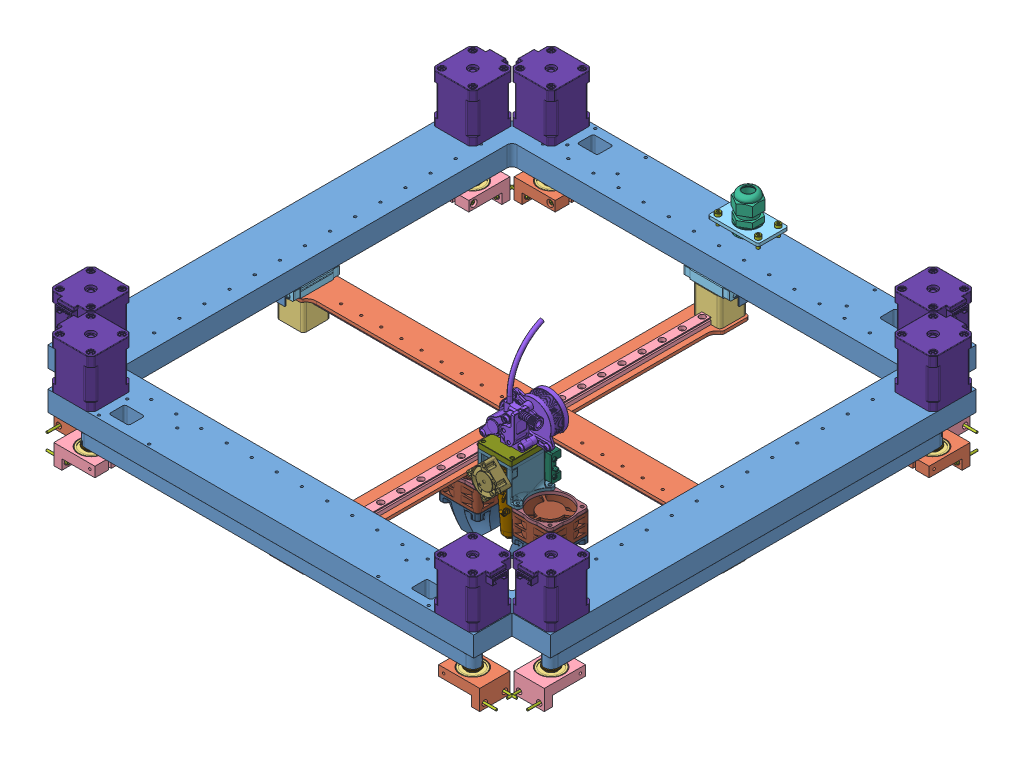
SolidWorks assembly ASM_Gantry_V3, configuration Default. Lengths in mm.
Overall size (500 178.35 500).
200 component instances, 28 part files, 43 mates.
Components (placement in the parent):
- PRT_Gantry_Main_Plate_V4-1: PRT_Gantry_Main_Plate_V4 [Default] at origin size (500 20 500)
- ASM_X_Beam_V1-3: ASM_X_Beam_V1 [Default] at (121.4512 212.7564 -330.8923) x (-1 0 0) z (0 0 1) size (442 41 48.55)
  - PRT_XY_Backer_V1-1: PRT_XY_Backer_V1 [Default] at (121.4512 223.2564 340.8937) size (442 3 38.2)
  - PRT_temp_backer_spacer-1: PRT_temp_backer_spacer [Default] at (328.9512 226.2564 330.8937) size (27 28 27)
  - PRT_temp_backer_spacer-2: PRT_temp_backer_spacer [Default] at (-86.0488 226.2564 330.8937) size (27 28 27)
  - PRT_MGN9H_Rail-2: PRT_MGN9H_Rail [400] at (-78.5488 229.5064 330.8937) x (0 0 -1) z (1 0 0) size (9 6.5 400)
  - PRT_MGN12H_Carriage-1: PRT_MGN12H_Carriage [Default] at (-86.0488 210.2564 314.6937) size (27 10 50.47)
  - PRT_MGN12H_Carriage-2: PRT_MGN12H_Carriage [Default] at (328.9512 210.2564 314.6937) size (27 10 50.47)
- ASM_Y_Beam_V1-1: ASM_Y_Beam_V1 [Default] at (-331.4877 -264.7564 121.4512) x (0 0 -1) z (1 0 0) size (442 41 48.55)
  - PRT_XY_Backer_V1-1: PRT_XY_Backer_V1 [Default] at (121.4512 223.2564 340.8937) size (442 3 38.2)
  - PRT_temp_backer_spacer-1: PRT_temp_backer_spacer [Default] at (328.9512 226.2564 330.8937) size (27 28 27)
  - PRT_temp_backer_spacer-2: PRT_temp_backer_spacer [Default] at (-86.0488 226.2564 330.8937) size (27 28 27)
  - PRT_MGN9H_Rail-2: PRT_MGN9H_Rail [400] at (-78.5488 229.5064 330.8937) x (0 0 -1) z (1 0 0) size (9 6.5 400)
  - PRT_MGN12H_Carriage-1: PRT_MGN12H_Carriage [Default] at (-86.0488 267.2564 314.6937) x (-1 0 0) z (0 0 1) size (27 10 50.47)
  - PRT_MGN12H_Carriage-2: PRT_MGN12H_Carriage [Default] at (328.9512 267.2564 314.6937) x (-1 0 0) z (0 0 1) size (27 10 50.47)
- ASM_Temp_Printhead_V1-1: ASM_Temp_Printhead_V1 [Default] at (-0.594 -28.5 21.5015) x (0 0 -1) z (1 0 0) size (54.33 135.01 54.33) (hidden)
  - PRT_Temp_Printhead_Plate_V1-1: PRT_Temp_Printhead_Plate_V1 [Default] at origin size (47 3 47)
  - PRT_MGN9H_Carriage-1: PRT_MGN9H_Carriage [По умолчанию] at (0 -4 0) x (0 0 1) z (-1 0 0) size (20 8 40.67)
  - PRT_MGN9H_Carriage-2: PRT_MGN9H_Carriage [По умолчанию] at (21.5 7 21.5) x (-1 0 0) z (0 0 1) size (20 8 40.67)
  - PRT_Chube_Integration-1: PRT_Chube_Integration [Default] at (-0.75 -32 22.25) x (1 0 0) z (0 -1 0) size (25.9 25.9 66.25)
  - PRT_Chube_Integration-2: PRT_Chube_Integration [Default] at (-0.75 35 22.25) x (-1 0 0) z (0 1 0) size (25.9 25.9 66.25) (hidden)
- ASM_MGN12_and_Screws_V1-1: ASM_MGN12_and_Screws_V1 [Default] at (35.6885 266.2419 374.1962) x (1 0 0) z (0 0 -1) size (12 14.5 360)
  - PRT_MGN12H_Rail-1: PRT_MGN12H_Rail [Default] at (165.8115 263.7419 208.1962) size (12 8 360)
  - socket head cap screw_am-1: socket head cap screw_am [B18.3.1M - 3 x 0.5 x 10 Hex SHCS -- 10NHX] at (171.8115 270.2419 550.6962) x (0 -1 0) z (0 0 1) size (13 5.5 5.5)
  - socket head cap screw_am-2: socket head cap screw_am [B18.3.1M - 3 x 0.5 x 10 Hex SHCS -- 10NHX] at (171.8115 270.2419 525.6962) x (0 -1 0) z (0 0 1) size (13 5.5 5.5)
  - socket head cap screw_am-3: socket head cap screw_am [B18.3.1M - 3 x 0.5 x 10 Hex SHCS -- 10NHX] at (171.8115 270.2419 500.6962) x (0 -1 0) z (0 0 1) size (13 5.5 5.5)
  - socket head cap screw_am-4: socket head cap screw_am [B18.3.1M - 3 x 0.5 x 10 Hex SHCS -- 10NHX] at (171.8115 270.2419 475.6962) x (0 -1 0) z (0 0 1) size (13 5.5 5.5)
  - socket head cap screw_am-5: socket head cap screw_am [B18.3.1M - 3 x 0.5 x 10 Hex SHCS -- 10NHX] at (171.8115 270.2419 450.6962) x (0 -1 0) z (0 0 1) size (13 5.5 5.5)
  - socket head cap screw_am-6: socket head cap screw_am [B18.3.1M - 3 x 0.5 x 10 Hex SHCS -- 10NHX] at (171.8115 270.2419 425.6962) x (0 -1 0) z (0 0 1) size (13 5.5 5.5)
  - socket head cap screw_am-7: socket head cap screw_am [B18.3.1M - 3 x 0.5 x 10 Hex SHCS -- 10NHX] at (171.8115 270.2419 400.6962) x (0 -1 0) z (0 0 1) size (13 5.5 5.5)
  - socket head cap screw_am-8: socket head cap screw_am [B18.3.1M - 3 x 0.5 x 10 Hex SHCS -- 10NHX] at (171.8115 270.2419 375.6962) x (0 -1 0) z (0 0 1) size (13 5.5 5.5)
  - socket head cap screw_am-9: socket head cap screw_am [B18.3.1M - 3 x 0.5 x 10 Hex SHCS -- 10NHX] at (171.8115 270.2419 350.6962) x (0 -1 0) z (0 0 1) size (13 5.5 5.5)
  - socket head cap screw_am-10: socket head cap screw_am [B18.3.1M - 3 x 0.5 x 10 Hex SHCS -- 10NHX] at (171.8115 270.2419 325.6962) x (0 -1 0) z (0 0 1) size (13 5.5 5.5)
  - socket head cap screw_am-11: socket head cap screw_am [B18.3.1M - 3 x 0.5 x 10 Hex SHCS -- 10NHX] at (171.8115 270.2419 300.6962) x (0 -1 0) z (0 0 1) size (13 5.5 5.5)
  - socket head cap screw_am-12: socket head cap screw_am [B18.3.1M - 3 x 0.5 x 10 Hex SHCS -- 10NHX] at (171.8115 270.2419 275.6962) x (0 -1 0) z (0 0 1) size (13 5.5 5.5)
  - socket head cap screw_am-13: socket head cap screw_am [B18.3.1M - 3 x 0.5 x 10 Hex SHCS -- 10NHX] at (171.8115 270.2419 250.6962) x (0 -1 0) z (0 0 1) size (13 5.5 5.5)
  - socket head cap screw_am-14: socket head cap screw_am [B18.3.1M - 3 x 0.5 x 10 Hex SHCS -- 10NHX] at (171.8115 270.2419 225.6962) x (0 -1 0) z (0 0 1) size (13 5.5 5.5)
- ASM_MGN12_and_Screws_V1-2: ASM_MGN12_and_Screws_V1 [Default] at (374.1962 266.2419 -35.6885) x (0 0 -1) z (-1 0 0) size (12 14.5 360)
  - PRT_MGN12H_Rail-1: PRT_MGN12H_Rail [Default] at (165.8115 263.7419 208.1962) size (12 8 360)
  - socket head cap screw_am-1: socket head cap screw_am [B18.3.1M - 3 x 0.5 x 10 Hex SHCS -- 10NHX] at (171.8115 270.2419 550.6962) x (0 -1 0) z (0 0 1) size (13 5.5 5.5)
  - socket head cap screw_am-2: socket head cap screw_am [B18.3.1M - 3 x 0.5 x 10 Hex SHCS -- 10NHX] at (171.8115 270.2419 525.6962) x (0 -1 0) z (0 0 1) size (13 5.5 5.5)
  - socket head cap screw_am-3: socket head cap screw_am [B18.3.1M - 3 x 0.5 x 10 Hex SHCS -- 10NHX] at (171.8115 270.2419 500.6962) x (0 -1 0) z (0 0 1) size (13 5.5 5.5)
  - socket head cap screw_am-4: socket head cap screw_am [B18.3.1M - 3 x 0.5 x 10 Hex SHCS -- 10NHX] at (171.8115 270.2419 475.6962) x (0 -1 0) z (0 0 1) size (13 5.5 5.5)
  - socket head cap screw_am-5: socket head cap screw_am [B18.3.1M - 3 x 0.5 x 10 Hex SHCS -- 10NHX] at (171.8115 270.2419 450.6962) x (0 -1 0) z (0 0 1) size (13 5.5 5.5)
  - socket head cap screw_am-6: socket head cap screw_am [B18.3.1M - 3 x 0.5 x 10 Hex SHCS -- 10NHX] at (171.8115 270.2419 425.6962) x (0 -1 0) z (0 0 1) size (13 5.5 5.5)
  - socket head cap screw_am-7: socket head cap screw_am [B18.3.1M - 3 x 0.5 x 10 Hex SHCS -- 10NHX] at (171.8115 270.2419 400.6962) x (0 -1 0) z (0 0 1) size (13 5.5 5.5)
  - socket head cap screw_am-8: socket head cap screw_am [B18.3.1M - 3 x 0.5 x 10 Hex SHCS -- 10NHX] at (171.8115 270.2419 375.6962) x (0 -1 0) z (0 0 1) size (13 5.5 5.5)
  - socket head cap screw_am-9: socket head cap screw_am [B18.3.1M - 3 x 0.5 x 10 Hex SHCS -- 10NHX] at (171.8115 270.2419 350.6962) x (0 -1 0) z (0 0 1) size (13 5.5 5.5)
  - socket head cap screw_am-10: socket head cap screw_am [B18.3.1M - 3 x 0.5 x 10 Hex SHCS -- 10NHX] at (171.8115 270.2419 325.6962) x (0 -1 0) z (0 0 1) size (13 5.5 5.5)
  - socket head cap screw_am-11: socket head cap screw_am [B18.3.1M - 3 x 0.5 x 10 Hex SHCS -- 10NHX] at (171.8115 270.2419 300.6962) x (0 -1 0) z (0 0 1) size (13 5.5 5.5)
  - socket head cap screw_am-12: socket head cap screw_am [B18.3.1M - 3 x 0.5 x 10 Hex SHCS -- 10NHX] at (171.8115 270.2419 275.6962) x (0 -1 0) z (0 0 1) size (13 5.5 5.5)
  - socket head cap screw_am-13: socket head cap screw_am [B18.3.1M - 3 x 0.5 x 10 Hex SHCS -- 10NHX] at (171.8115 270.2419 250.6962) x (0 -1 0) z (0 0 1) size (13 5.5 5.5)
  - socket head cap screw_am-14: socket head cap screw_am [B18.3.1M - 3 x 0.5 x 10 Hex SHCS -- 10NHX] at (171.8115 270.2419 225.6962) x (0 -1 0) z (0 0 1) size (13 5.5 5.5)
- ASM_MGN12_and_Screws_V1-3: ASM_MGN12_and_Screws_V1 [Default] at (-379.3115 266.2419 374.1962) x (1 0 0) z (0 0 -1) size (12 14.5 360)
  - PRT_MGN12H_Rail-1: PRT_MGN12H_Rail [Default] at (165.8115 263.7419 208.1962) size (12 8 360)
  - socket head cap screw_am-1: socket head cap screw_am [B18.3.1M - 3 x 0.5 x 10 Hex SHCS -- 10NHX] at (171.8115 270.2419 550.6962) x (0 -1 0) z (0 0 1) size (13 5.5 5.5)
  - socket head cap screw_am-2: socket head cap screw_am [B18.3.1M - 3 x 0.5 x 10 Hex SHCS -- 10NHX] at (171.8115 270.2419 525.6962) x (0 -1 0) z (0 0 1) size (13 5.5 5.5)
  - socket head cap screw_am-3: socket head cap screw_am [B18.3.1M - 3 x 0.5 x 10 Hex SHCS -- 10NHX] at (171.8115 270.2419 500.6962) x (0 -1 0) z (0 0 1) size (13 5.5 5.5)
  - socket head cap screw_am-4: socket head cap screw_am [B18.3.1M - 3 x 0.5 x 10 Hex SHCS -- 10NHX] at (171.8115 270.2419 475.6962) x (0 -1 0) z (0 0 1) size (13 5.5 5.5)
  - socket head cap screw_am-5: socket head cap screw_am [B18.3.1M - 3 x 0.5 x 10 Hex SHCS -- 10NHX] at (171.8115 270.2419 450.6962) x (0 -1 0) z (0 0 1) size (13 5.5 5.5)
  - socket head cap screw_am-6: socket head cap screw_am [B18.3.1M - 3 x 0.5 x 10 Hex SHCS -- 10NHX] at (171.8115 270.2419 425.6962) x (0 -1 0) z (0 0 1) size (13 5.5 5.5)
  - socket head cap screw_am-7: socket head cap screw_am [B18.3.1M - 3 x 0.5 x 10 Hex SHCS -- 10NHX] at (171.8115 270.2419 400.6962) x (0 -1 0) z (0 0 1) size (13 5.5 5.5)
  - socket head cap screw_am-8: socket head cap screw_am [B18.3.1M - 3 x 0.5 x 10 Hex SHCS -- 10NHX] at (171.8115 270.2419 375.6962) x (0 -1 0) z (0 0 1) size (13 5.5 5.5)
  - socket head cap screw_am-9: socket head cap screw_am [B18.3.1M - 3 x 0.5 x 10 Hex SHCS -- 10NHX] at (171.8115 270.2419 350.6962) x (0 -1 0) z (0 0 1) size (13 5.5 5.5)
  - socket head cap screw_am-10: socket head cap screw_am [B18.3.1M - 3 x 0.5 x 10 Hex SHCS -- 10NHX] at (171.8115 270.2419 325.6962) x (0 -1 0) z (0 0 1) size (13 5.5 5.5)
  - socket head cap screw_am-11: socket head cap screw_am [B18.3.1M - 3 x 0.5 x 10 Hex SHCS -- 10NHX] at (171.8115 270.2419 300.6962) x (0 -1 0) z (0 0 1) size (13 5.5 5.5)
  - socket head cap screw_am-12: socket head cap screw_am [B18.3.1M - 3 x 0.5 x 10 Hex SHCS -- 10NHX] at (171.8115 270.2419 275.6962) x (0 -1 0) z (0 0 1) size (13 5.5 5.5)
  - socket head cap screw_am-13: socket head cap screw_am [B18.3.1M - 3 x 0.5 x 10 Hex SHCS -- 10NHX] at (171.8115 270.2419 250.6962) x (0 -1 0) z (0 0 1) size (13 5.5 5.5)
  - socket head cap screw_am-14: socket head cap screw_am [B18.3.1M - 3 x 0.5 x 10 Hex SHCS -- 10NHX] at (171.8115 270.2419 225.6962) x (0 -1 0) z (0 0 1) size (13 5.5 5.5)
- ASM_MGN12_and_Screws_V1-4: ASM_MGN12_and_Screws_V1 [Default] at (-402.1962 266.2419 35.6885) x (0 0 1) z (1 0 0) size (12 14.5 360)
  - PRT_MGN12H_Rail-1: PRT_MGN12H_Rail [Default] at (165.8115 263.7419 208.1962) size (12 8 360)
  - socket head cap screw_am-1: socket head cap screw_am [B18.3.1M - 3 x 0.5 x 10 Hex SHCS -- 10NHX] at (171.8115 270.2419 550.6962) x (0 -1 0) z (0 0 1) size (13 5.5 5.5)
  - socket head cap screw_am-2: socket head cap screw_am [B18.3.1M - 3 x 0.5 x 10 Hex SHCS -- 10NHX] at (171.8115 270.2419 525.6962) x (0 -1 0) z (0 0 1) size (13 5.5 5.5)
  - socket head cap screw_am-3: socket head cap screw_am [B18.3.1M - 3 x 0.5 x 10 Hex SHCS -- 10NHX] at (171.8115 270.2419 500.6962) x (0 -1 0) z (0 0 1) size (13 5.5 5.5)
  - socket head cap screw_am-4: socket head cap screw_am [B18.3.1M - 3 x 0.5 x 10 Hex SHCS -- 10NHX] at (171.8115 270.2419 475.6962) x (0 -1 0) z (0 0 1) size (13 5.5 5.5)
  - socket head cap screw_am-5: socket head cap screw_am [B18.3.1M - 3 x 0.5 x 10 Hex SHCS -- 10NHX] at (171.8115 270.2419 450.6962) x (0 -1 0) z (0 0 1) size (13 5.5 5.5)
  - socket head cap screw_am-6: socket head cap screw_am [B18.3.1M - 3 x 0.5 x 10 Hex SHCS -- 10NHX] at (171.8115 270.2419 425.6962) x (0 -1 0) z (0 0 1) size (13 5.5 5.5)
  - socket head cap screw_am-7: socket head cap screw_am [B18.3.1M - 3 x 0.5 x 10 Hex SHCS -- 10NHX] at (171.8115 270.2419 400.6962) x (0 -1 0) z (0 0 1) size (13 5.5 5.5)
  - socket head cap screw_am-8: socket head cap screw_am [B18.3.1M - 3 x 0.5 x 10 Hex SHCS -- 10NHX] at (171.8115 270.2419 375.6962) x (0 -1 0) z (0 0 1) size (13 5.5 5.5)
  - socket head cap screw_am-9: socket head cap screw_am [B18.3.1M - 3 x 0.5 x 10 Hex SHCS -- 10NHX] at (171.8115 270.2419 350.6962) x (0 -1 0) z (0 0 1) size (13 5.5 5.5)
  - socket head cap screw_am-10: socket head cap screw_am [B18.3.1M - 3 x 0.5 x 10 Hex SHCS -- 10NHX] at (171.8115 270.2419 325.6962) x (0 -1 0) z (0 0 1) size (13 5.5 5.5)
  - socket head cap screw_am-11: socket head cap screw_am [B18.3.1M - 3 x 0.5 x 10 Hex SHCS -- 10NHX] at (171.8115 270.2419 300.6962) x (0 -1 0) z (0 0 1) size (13 5.5 5.5)
  - socket head cap screw_am-12: socket head cap screw_am [B18.3.1M - 3 x 0.5 x 10 Hex SHCS -- 10NHX] at (171.8115 270.2419 275.6962) x (0 -1 0) z (0 0 1) size (13 5.5 5.5)
  - socket head cap screw_am-13: socket head cap screw_am [B18.3.1M - 3 x 0.5 x 10 Hex SHCS -- 10NHX] at (171.8115 270.2419 250.6962) x (0 -1 0) z (0 0 1) size (13 5.5 5.5)
  - socket head cap screw_am-14: socket head cap screw_am [B18.3.1M - 3 x 0.5 x 10 Hex SHCS -- 10NHX] at (171.8115 270.2419 225.6962) x (0 -1 0) z (0 0 1) size (13 5.5 5.5)
- Assem - Printhead v2-1: Assem - Printhead v2 [Default] at (37.6705 -41.0301 26.4666) size (113.64 178.35 58.81)
  - Vz-Hextrudort CNC-1: Vz-Hextrudort CNC [Default] at (-15.7303 41.095 -9.5652) x (1 0 0) z (0 1 0) size (52.06 45.53 91.4)
  - Goliath Mockup AIR-1: Goliath Mockup AIR [Default] at (-11.4303 -33.3199 1.9348) x (0 0 -1) z (0 1 0) size (33.99 25.16 69.25)
  - Tiger Fan Duct-1: Tiger Fan Duct [Default] at (-11.4303 -73.3179 1.9348) x (0 0 1) z (-1 0 0) size (51.43 33.95 113.41)
  - 40x20 fan-2: 40x20 fan [По умолчанию] at (24.5697 -38.9699 -2.0652) x (-1 0 0) z (0 1 0) size (41.13 41.33 20.18)
  - 40x20 fan-1: 40x20 fan [По умолчанию] at (-47.4303 -38.9699 -2.0652) x (-1 0 0) z (0 1 0) size (41.13 41.33 20.18)
  - Fan Mount Top-1: Fan Mount Top [Default] at (-11.4303 -13.9699 1.9348) x (-1 0 0) z (0 -1 0) size (114.33 42.33 12.5) (hidden)
  - 25x25x10 Fan-1: 25x25x10 Fan [Default] at (-11.4303 2.3051 17.4624) x (0.707107 -0.707107 0) z (0 0 1) size (25.78 25.81 10.5)
  - Fan Mount Top Alu-1: Fan Mount Top Alu [Default] at (-11.4303 -18.9699 1.9348) x (1 0 0) z (0 1 0) size (113.33 41.33 3)
  - Chassis 3DP-1: Chassis 3DP [Default] at (-11.4303 -15.9699 1.9348) x (1 0 0) z (0 1 0) size (47.06 39.07 34.15)
  - x_mgn12_h_carriage-1: x_mgn12_h_carriage [Default] at (-27.6303 2.0301 -29.4652) x (0 1 0) z (1 0 0) size (27 10 50.47)
  - Extruder Mount-1: Extruder Mount [Default] at (-11.4303 18.1801 1.9348) x (1 0 0) z (0 1 0) size (33.67 33.93 5)
- ASM_XY_Transmission_V1-1: ASM_XY_Transmission_V1 [Default] at (-163.4074 -55.5632 126.4064) size (447.8 117 42)
  - PRT_LDO-42STH48-2504AHS8-55-1: PRT_LDO-42STH48-2504AHS8-55 [Default] at (-26.5926 116.0632 102.5936) x (0 0 -1) z (-1 0 0) size (42 103 48.25)
  - PRT_LDO-42STH48-2504AHS8-55-2: PRT_LDO-42STH48-2504AHS8-55 [Default] at (353.4074 116.0632 102.5936) x (0 0 1) z (1 0 0) size (42 103 48.25)
  - PRT_Gates_2GT_20T_Toothed_Pulley_12mm_8mm-Bore-1: PRT_Gates_2GT_20T_Toothed_Pulley_12mm_8mm-Bore [Výchozí] at (-26.5926 49.5632 102.5936) x (0 0 1) z (1 0 0) size (15 22 15)
  - PRT_Gates_2GT_20T_Toothed_Pulley_12mm_8mm-Bore-2: PRT_Gates_2GT_20T_Toothed_Pulley_12mm_8mm-Bore [Výchozí] at (353.4074 49.5632 102.5936) x (0 0 1) z (1 0 0) size (15 22 15)
  - PRT_XY_Belt_Path_V1-1: PRT_XY_Belt_Path_V1 [Default] at (353.4074 29.2632 102.5936) x (-1 0 0) z (0 0 -1) size (393.48 12 24.44)
  - ASM_Bearing_Block_8mm_V1-1: ASM_Bearing_Block_8mm_V1 [Default] at (341.4747 43.8938 139.9297) x (1 0 0) z (0 0 -1) size (52.9 20 30)
    - PRT_Bearing_Block_8mm_V1-1: PRT_Bearing_Block_8mm_V1 [Default] at (11.9326 17.3307 37.3361) x (0 0 -1) z (0 1 0) size (30 40.9 20)
    - socket head cap screw_am-1: socket head cap screw_am [B18.3.1M - 2 x 0.4 x 20 Hex SHCS -- 16NHX] at (23.8326 32.3307 47.3361) size (22 3.8 3.8)
    - socket head cap screw_am-2: socket head cap screw_am [B18.3.1M - 2 x 0.4 x 20 Hex SHCS -- 16NHX] at (23.8326 32.3307 27.3361) size (22 3.8 3.8)
    - socket head cap screw_am-3: socket head cap screw_am [B18.3.1M - 2 x 0.4 x 20 Hex SHCS -- 16NHX] at (-2.0674 22.3307 51.3361) x (0 0 -1) z (1 0 0) size (22 3.8 3.8)
    - PRT_SB628ZZ_Bearing-2: PRT_SB628ZZ_Bearing [Default] at (11.9326 17.3307 37.3361) x (0 1 0) z (0.078254 0 0.996933) size (8 24 24)
  - ASM_Bearing_Block_8mm_Mirror_V1-1: ASM_Bearing_Block_8mm_Mirror_V1 [Default] at (-18.8216 41.3233 61.3151) x (-1 0 0) z (0 0 1) size (52.9 20 30)
    - PRT_Bearing_Block_8mm_Mirror_V1-1: PRT_Bearing_Block_8mm_Mirror_V1 [Default] at (7.771 14.7602 41.2785) x (0 0 -1) z (0 1 0) size (30 40.9 20)
    - socket head cap screw_am-1: socket head cap screw_am [B18.3.1M - 2 x 0.4 x 20 Hex SHCS -- 16NHX] at (19.671 29.7602 31.2785) size (22 3.8 3.8)
    - socket head cap screw_am-2: socket head cap screw_am [B18.3.1M - 2 x 0.4 x 20 Hex SHCS -- 16NHX] at (19.671 29.7602 51.2785) size (22 3.8 3.8)
    - socket head cap screw_am-3: socket head cap screw_am [B18.3.1M - 2 x 0.4 x 20 Hex SHCS -- 16NHX] at (-6.229 19.7602 27.2785) x (0 0 1) z (-1 0 0) size (22 3.8 3.8)
    - PRT_SB628ZZ_Bearing-1: PRT_SB628ZZ_Bearing [Default] at (7.771 14.7602 41.2785) x (0 1 0) z (-0.143467 0 0.989655) size (8 24 24)
  - socket head cap screw_am-1: socket head cap screw_am [B18.3.1M - 2 x 0.4 x 20 Hex SHCS -- 16NHX] at (-42.0946 53.5632 118.0956) x (0 1 0) z (-0.989891 0 0.141832) size (22 3.8 3.8)
  - socket head cap screw_am-2: socket head cap screw_am [B18.3.1M - 2 x 0.4 x 20 Hex SHCS -- 16NHX] at (-11.0907 53.5632 118.0956) x (0 1 0) z (-0.998853 0 -0.047874) size (22 3.8 3.8)
  - socket head cap screw_am-4: socket head cap screw_am [B18.3.1M - 2 x 0.4 x 20 Hex SHCS -- 16NHX] at (368.9093 53.5632 87.0917) x (0 1 0) z (-0.40555 0 0.914073) size (22 3.8 3.8)
  - socket head cap screw_am-5: socket head cap screw_am [B18.3.1M - 2 x 0.4 x 20 Hex SHCS -- 16NHX] at (368.9093 53.5632 118.0956) x (0 1 0) z (-0.40555 0 0.914073) size (22 3.8 3.8)
  - socket head cap screw_am-6: socket head cap screw_am [B18.3.1M - 2 x 0.4 x 20 Hex SHCS -- 16NHX] at (337.9054 53.5632 118.0956) x (0 1 0) z (-0.40555 0 0.914073) size (22 3.8 3.8)
  - socket head cap screw_am-7: socket head cap screw_am [B18.3.1M - 2 x 0.4 x 20 Hex SHCS -- 16NHX] at (-42.0946 53.5632 87.0917) x (0 1 0) z (-0.40555 0 0.914073) size (22 3.8 3.8)
- ASM_XY_Transmission_V1-2: ASM_XY_Transmission_V1 [Default] at (126.4064 -55.5632 163.4074) x (0 0 -1) z (1 0 0) size (447.8 117 42)
  - PRT_LDO-42STH48-2504AHS8-55-1: PRT_LDO-42STH48-2504AHS8-55 [Default] at (-26.5926 116.0632 102.5936) x (0 0 -1) z (-1 0 0) size (42 103 48.25)
  - PRT_LDO-42STH48-2504AHS8-55-2: PRT_LDO-42STH48-2504AHS8-55 [Default] at (353.4074 116.0632 102.5936) x (0 0 1) z (1 0 0) size (42 103 48.25)
  - PRT_Gates_2GT_20T_Toothed_Pulley_12mm_8mm-Bore-1: PRT_Gates_2GT_20T_Toothed_Pulley_12mm_8mm-Bore [Výchozí] at (-26.5926 49.5632 102.5936) x (0 0 1) z (1 0 0) size (15 22 15)
  - PRT_Gates_2GT_20T_Toothed_Pulley_12mm_8mm-Bore-2: PRT_Gates_2GT_20T_Toothed_Pulley_12mm_8mm-Bore [Výchozí] at (353.4074 49.5632 102.5936) x (0 0 1) z (1 0 0) size (15 22 15)
  - PRT_XY_Belt_Path_V1-1: PRT_XY_Belt_Path_V1 [Default] at (353.4074 29.2632 102.5936) x (-1 0 0) z (0 0 -1) size (393.48 12 24.44)
  - ASM_Bearing_Block_8mm_V1-1: ASM_Bearing_Block_8mm_V1 [Default] at (341.4747 43.8938 139.9297) x (1 0 0) z (0 0 -1) size (52.9 20 30)
    - PRT_Bearing_Block_8mm_V1-1: PRT_Bearing_Block_8mm_V1 [Default] at (11.9326 17.3307 37.3361) x (0 0 -1) z (0 1 0) size (30 40.9 20)
    - socket head cap screw_am-1: socket head cap screw_am [B18.3.1M - 2 x 0.4 x 20 Hex SHCS -- 16NHX] at (23.8326 32.3307 47.3361) size (22 3.8 3.8)
    - socket head cap screw_am-2: socket head cap screw_am [B18.3.1M - 2 x 0.4 x 20 Hex SHCS -- 16NHX] at (23.8326 32.3307 27.3361) size (22 3.8 3.8)
    - socket head cap screw_am-3: socket head cap screw_am [B18.3.1M - 2 x 0.4 x 20 Hex SHCS -- 16NHX] at (-2.0674 22.3307 51.3361) x (0 0 -1) z (1 0 0) size (22 3.8 3.8)
    - PRT_SB628ZZ_Bearing-2: PRT_SB628ZZ_Bearing [Default] at (11.9326 17.3307 37.3361) x (0 1 0) z (0.078254 0 0.996933) size (8 24 24)
  - ASM_Bearing_Block_8mm_Mirror_V1-1: ASM_Bearing_Block_8mm_Mirror_V1 [Default] at (-18.8216 41.3233 61.3151) x (-1 0 0) z (0 0 1) size (52.9 20 30)
    - PRT_Bearing_Block_8mm_Mirror_V1-1: PRT_Bearing_Block_8mm_Mirror_V1 [Default] at (7.771 14.7602 41.2785) x (0 0 -1) z (0 1 0) size (30 40.9 20)
    - socket head cap screw_am-1: socket head cap screw_am [B18.3.1M - 2 x 0.4 x 20 Hex SHCS -- 16NHX] at (19.671 29.7602 31.2785) size (22 3.8 3.8)
    - socket head cap screw_am-2: socket head cap screw_am [B18.3.1M - 2 x 0.4 x 20 Hex SHCS -- 16NHX] at (19.671 29.7602 51.2785) size (22 3.8 3.8)
    - socket head cap screw_am-3: socket head cap screw_am [B18.3.1M - 2 x 0.4 x 20 Hex SHCS -- 16NHX] at (-6.229 19.7602 27.2785) x (0 0 1) z (-1 0 0) size (22 3.8 3.8)
    - PRT_SB628ZZ_Bearing-1: PRT_SB628ZZ_Bearing [Default] at (7.771 14.7602 41.2785) x (0 1 0) z (-0.143467 0 0.989655) size (8 24 24)
  - socket head cap screw_am-1: socket head cap screw_am [B18.3.1M - 2 x 0.4 x 20 Hex SHCS -- 16NHX] at (-42.0946 53.5632 118.0956) x (0 1 0) z (-0.989891 0 0.141832) size (22 3.8 3.8)
  - socket head cap screw_am-2: socket head cap screw_am [B18.3.1M - 2 x 0.4 x 20 Hex SHCS -- 16NHX] at (-11.0907 53.5632 118.0956) x (0 1 0) z (-0.998853 0 -0.047874) size (22 3.8 3.8)
  - socket head cap screw_am-4: socket head cap screw_am [B18.3.1M - 2 x 0.4 x 20 Hex SHCS -- 16NHX] at (368.9093 53.5632 87.0917) x (0 1 0) z (-0.40555 0 0.914073) size (22 3.8 3.8)
  - socket head cap screw_am-5: socket head cap screw_am [B18.3.1M - 2 x 0.4 x 20 Hex SHCS -- 16NHX] at (368.9093 53.5632 118.0956) x (0 1 0) z (-0.40555 0 0.914073) size (22 3.8 3.8)
  - socket head cap screw_am-6: socket head cap screw_am [B18.3.1M - 2 x 0.4 x 20 Hex SHCS -- 16NHX] at (337.9054 53.5632 118.0956) x (0 1 0) z (-0.40555 0 0.914073) size (22 3.8 3.8)
  - socket head cap screw_am-7: socket head cap screw_am [B18.3.1M - 2 x 0.4 x 20 Hex SHCS -- 16NHX] at (-42.0946 53.5632 87.0917) x (0 1 0) z (-0.40555 0 0.914073) size (22 3.8 3.8)
- ASM_XY_Transmission_V1-3: ASM_XY_Transmission_V1 [Default] at (163.4074 -55.5632 -126.4064) x (-1 0 0) z (0 0 -1) size (447.8 117 42)
  - PRT_LDO-42STH48-2504AHS8-55-1: PRT_LDO-42STH48-2504AHS8-55 [Default] at (-26.5926 116.0632 102.5936) x (0 0 -1) z (-1 0 0) size (42 103 48.25)
  - PRT_LDO-42STH48-2504AHS8-55-2: PRT_LDO-42STH48-2504AHS8-55 [Default] at (353.4074 116.0632 102.5936) x (0 0 1) z (1 0 0) size (42 103 48.25)
  - PRT_Gates_2GT_20T_Toothed_Pulley_12mm_8mm-Bore-1: PRT_Gates_2GT_20T_Toothed_Pulley_12mm_8mm-Bore [Výchozí] at (-26.5926 49.5632 102.5936) x (0 0 1) z (1 0 0) size (15 22 15)
  - PRT_Gates_2GT_20T_Toothed_Pulley_12mm_8mm-Bore-2: PRT_Gates_2GT_20T_Toothed_Pulley_12mm_8mm-Bore [Výchozí] at (353.4074 49.5632 102.5936) x (0 0 1) z (1 0 0) size (15 22 15)
  - PRT_XY_Belt_Path_V1-1: PRT_XY_Belt_Path_V1 [Default] at (353.4074 29.2632 102.5936) x (-1 0 0) z (0 0 -1) size (393.48 12 24.44)
  - ASM_Bearing_Block_8mm_V1-1: ASM_Bearing_Block_8mm_V1 [Default] at (341.4747 43.8938 139.9297) x (1 0 0) z (0 0 -1) size (52.9 20 30)
    - PRT_Bearing_Block_8mm_V1-1: PRT_Bearing_Block_8mm_V1 [Default] at (11.9326 17.3307 37.3361) x (0 0 -1) z (0 1 0) size (30 40.9 20)
    - socket head cap screw_am-1: socket head cap screw_am [B18.3.1M - 2 x 0.4 x 20 Hex SHCS -- 16NHX] at (23.8326 32.3307 47.3361) size (22 3.8 3.8)
    - socket head cap screw_am-2: socket head cap screw_am [B18.3.1M - 2 x 0.4 x 20 Hex SHCS -- 16NHX] at (23.8326 32.3307 27.3361) size (22 3.8 3.8)
    - socket head cap screw_am-3: socket head cap screw_am [B18.3.1M - 2 x 0.4 x 20 Hex SHCS -- 16NHX] at (-2.0674 22.3307 51.3361) x (0 0 -1) z (1 0 0) size (22 3.8 3.8)
    - PRT_SB628ZZ_Bearing-2: PRT_SB628ZZ_Bearing [Default] at (11.9326 17.3307 37.3361) x (0 1 0) z (0.078254 0 0.996933) size (8 24 24)
  - ASM_Bearing_Block_8mm_Mirror_V1-1: ASM_Bearing_Block_8mm_Mirror_V1 [Default] at (-18.8216 41.3233 61.3151) x (-1 0 0) z (0 0 1) size (52.9 20 30)
    - PRT_Bearing_Block_8mm_Mirror_V1-1: PRT_Bearing_Block_8mm_Mirror_V1 [Default] at (7.771 14.7602 41.2785) x (0 0 -1) z (0 1 0) size (30 40.9 20)
    - socket head cap screw_am-1: socket head cap screw_am [B18.3.1M - 2 x 0.4 x 20 Hex SHCS -- 16NHX] at (19.671 29.7602 31.2785) size (22 3.8 3.8)
    - socket head cap screw_am-2: socket head cap screw_am [B18.3.1M - 2 x 0.4 x 20 Hex SHCS -- 16NHX] at (19.671 29.7602 51.2785) size (22 3.8 3.8)
    - socket head cap screw_am-3: socket head cap screw_am [B18.3.1M - 2 x 0.4 x 20 Hex SHCS -- 16NHX] at (-6.229 19.7602 27.2785) x (0 0 1) z (-1 0 0) size (22 3.8 3.8)
    - PRT_SB628ZZ_Bearing-1: PRT_SB628ZZ_Bearing [Default] at (7.771 14.7602 41.2785) x (0 1 0) z (-0.143467 0 0.989655) size (8 24 24)
  - socket head cap screw_am-1: socket head cap screw_am [B18.3.1M - 2 x 0.4 x 20 Hex SHCS -- 16NHX] at (-42.0946 53.5632 118.0956) x (0 1 0) z (-0.989891 0 0.141832) size (22 3.8 3.8)
  - socket head cap screw_am-2: socket head cap screw_am [B18.3.1M - 2 x 0.4 x 20 Hex SHCS -- 16NHX] at (-11.0907 53.5632 118.0956) x (0 1 0) z (-0.998853 0 -0.047874) size (22 3.8 3.8)
  - socket head cap screw_am-4: socket head cap screw_am [B18.3.1M - 2 x 0.4 x 20 Hex SHCS -- 16NHX] at (368.9093 53.5632 87.0917) x (0 1 0) z (-0.40555 0 0.914073) size (22 3.8 3.8)
  - socket head cap screw_am-5: socket head cap screw_am [B18.3.1M - 2 x 0.4 x 20 Hex SHCS -- 16NHX] at (368.9093 53.5632 118.0956) x (0 1 0) z (-0.40555 0 0.914073) size (22 3.8 3.8)
  - socket head cap screw_am-6: socket head cap screw_am [B18.3.1M - 2 x 0.4 x 20 Hex SHCS -- 16NHX] at (337.9054 53.5632 118.0956) x (0 1 0) z (-0.40555 0 0.914073) size (22 3.8 3.8)
  - socket head cap screw_am-7: socket head cap screw_am [B18.3.1M - 2 x 0.4 x 20 Hex SHCS -- 16NHX] at (-42.0946 53.5632 87.0917) x (0 1 0) z (-0.40555 0 0.914073) size (22 3.8 3.8)
- ASM_XY_Transmission_V1-4: ASM_XY_Transmission_V1 [Default] at (-126.4064 -55.5632 -163.4074) x (0 0 1) z (-1 0 0) size (447.8 117 42)
  - PRT_LDO-42STH48-2504AHS8-55-1: PRT_LDO-42STH48-2504AHS8-55 [Default] at (-26.5926 116.0632 102.5936) x (0 0 -1) z (-1 0 0) size (42 103 48.25)
  - PRT_LDO-42STH48-2504AHS8-55-2: PRT_LDO-42STH48-2504AHS8-55 [Default] at (353.4074 116.0632 102.5936) x (0 0 1) z (1 0 0) size (42 103 48.25)
  - PRT_Gates_2GT_20T_Toothed_Pulley_12mm_8mm-Bore-1: PRT_Gates_2GT_20T_Toothed_Pulley_12mm_8mm-Bore [Výchozí] at (-26.5926 49.5632 102.5936) x (0 0 1) z (1 0 0) size (15 22 15)
  - PRT_Gates_2GT_20T_Toothed_Pulley_12mm_8mm-Bore-2: PRT_Gates_2GT_20T_Toothed_Pulley_12mm_8mm-Bore [Výchozí] at (353.4074 49.5632 102.5936) x (0 0 1) z (1 0 0) size (15 22 15)
  - PRT_XY_Belt_Path_V1-1: PRT_XY_Belt_Path_V1 [Default] at (353.4074 29.2632 102.5936) x (-1 0 0) z (0 0 -1) size (393.48 12 24.44)
  - ASM_Bearing_Block_8mm_V1-1: ASM_Bearing_Block_8mm_V1 [Default] at (341.4747 43.8938 139.9297) x (1 0 0) z (0 0 -1) size (52.9 20 30)
    - PRT_Bearing_Block_8mm_V1-1: PRT_Bearing_Block_8mm_V1 [Default] at (11.9326 17.3307 37.3361) x (0 0 -1) z (0 1 0) size (30 40.9 20)
    - socket head cap screw_am-1: socket head cap screw_am [B18.3.1M - 2 x 0.4 x 20 Hex SHCS -- 16NHX] at (23.8326 32.3307 47.3361) size (22 3.8 3.8)
    - socket head cap screw_am-2: socket head cap screw_am [B18.3.1M - 2 x 0.4 x 20 Hex SHCS -- 16NHX] at (23.8326 32.3307 27.3361) size (22 3.8 3.8)
    - socket head cap screw_am-3: socket head cap screw_am [B18.3.1M - 2 x 0.4 x 20 Hex SHCS -- 16NHX] at (-2.0674 22.3307 51.3361) x (0 0 -1) z (1 0 0) size (22 3.8 3.8)
    - PRT_SB628ZZ_Bearing-2: PRT_SB628ZZ_Bearing [Default] at (11.9326 17.3307 37.3361) x (0 1 0) z (0.078254 0 0.996933) size (8 24 24)
  - ASM_Bearing_Block_8mm_Mirror_V1-1: ASM_Bearing_Block_8mm_Mirror_V1 [Default] at (-18.8216 41.3233 61.3151) x (-1 0 0) z (0 0 1) size (52.9 20 30)
    - PRT_Bearing_Block_8mm_Mirror_V1-1: PRT_Bearing_Block_8mm_Mirror_V1 [Default] at (7.771 14.7602 41.2785) x (0 0 -1) z (0 1 0) size (30 40.9 20)
    - socket head cap screw_am-1: socket head cap screw_am [B18.3.1M - 2 x 0.4 x 20 Hex SHCS -- 16NHX] at (19.671 29.7602 31.2785) size (22 3.8 3.8)
    - socket head cap screw_am-2: socket head cap screw_am [B18.3.1M - 2 x 0.4 x 20 Hex SHCS -- 16NHX] at (19.671 29.7602 51.2785) size (22 3.8 3.8)
    - socket head cap screw_am-3: socket head cap screw_am [B18.3.1M - 2 x 0.4 x 20 Hex SHCS -- 16NHX] at (-6.229 19.7602 27.2785) x (0 0 1) z (-1 0 0) size (22 3.8 3.8)
    - PRT_SB628ZZ_Bearing-1: PRT_SB628ZZ_Bearing [Default] at (7.771 14.7602 41.2785) x (0 1 0) z (-0.143467 0 0.989655) size (8 24 24)
  - socket head cap screw_am-1: socket head cap screw_am [B18.3.1M - 2 x 0.4 x 20 Hex SHCS -- 16NHX] at (-42.0946 53.5632 118.0956) x (0 1 0) z (-0.989891 0 0.141832) size (22 3.8 3.8)
  - socket head cap screw_am-2: socket head cap screw_am [B18.3.1M - 2 x 0.4 x 20 Hex SHCS -- 16NHX] at (-11.0907 53.5632 118.0956) x (0 1 0) z (-0.998853 0 -0.047874) size (22 3.8 3.8)
  - socket head cap screw_am-4: socket head cap screw_am [B18.3.1M - 2 x 0.4 x 20 Hex SHCS -- 16NHX] at (368.9093 53.5632 87.0917) x (0 1 0) z (-0.40555 0 0.914073) size (22 3.8 3.8)
  - socket head cap screw_am-5: socket head cap screw_am [B18.3.1M - 2 x 0.4 x 20 Hex SHCS -- 16NHX] at (368.9093 53.5632 118.0956) x (0 1 0) z (-0.40555 0 0.914073) size (22 3.8 3.8)
  - socket head cap screw_am-6: socket head cap screw_am [B18.3.1M - 2 x 0.4 x 20 Hex SHCS -- 16NHX] at (337.9054 53.5632 118.0956) x (0 1 0) z (-0.40555 0 0.914073) size (22 3.8 3.8)
  - socket head cap screw_am-7: socket head cap screw_am [B18.3.1M - 2 x 0.4 x 20 Hex SHCS -- 16NHX] at (-42.0946 53.5632 87.0917) x (0 1 0) z (-0.40555 0 0.914073) size (22 3.8 3.8)
- ASM_PG11_Mount_V1-1: ASM_PG11_Mount_V1 [Default] at (-20.8322 -2.2726 -271.0258) size (50 38.77 30)
  - PRT_PG11_Mount_V1-1: PRT_PG11_Mount_V1 [Default] at (20.8322 27.8726 36.0258) size (50 3 30)
  - PRT_PG11_Gland-1: PRT_PG11_Gland [Default] at (20.8322 31.7726 36.0258) x (1 0 0) z (0 1 0) size (24 26.25 35.37)
  - socket head cap screw_am-1: socket head cap screw_am [B18.3.1M - 3 x 0.5 x 12 Hex SHCS -- 12NHX] at (0.8322 33.8726 46.0258) x (0 -1 0) z (0 0 1) size (15 5.5 5.5)
  - socket head cap screw_am-2: socket head cap screw_am [B18.3.1M - 3 x 0.5 x 12 Hex SHCS -- 12NHX] at (0.8322 33.8726 26.0258) x (0 -1 0) z (0 0 1) size (15 5.5 5.5)
  - socket head cap screw_am-3: socket head cap screw_am [B18.3.1M - 3 x 0.5 x 12 Hex SHCS -- 12NHX] at (40.8322 33.8726 26.0258) x (0 -1 0) z (0 0 1) size (15 5.5 5.5)
  - socket head cap screw_am-4: socket head cap screw_am [B18.3.1M - 3 x 0.5 x 12 Hex SHCS -- 12NHX] at (40.8322 33.8726 46.0258) x (0 -1 0) z (0 0 1) size (15 5.5 5.5)
Mates (geometry in assembly coordinates):
- Coincident16: coincident aligned: plane of PRT_Gantry_Main_Plate_V4-1 through (0 0 0) normal (0 0 1)
- Coincident17: coincident aligned: plane of PRT_Gantry_Main_Plate_V4-1 through (0 0 0) normal (0 1 0)
- Coincident18: coincident aligned: plane of PRT_Gantry_Main_Plate_V4-1 through (0 0 0) normal (1 0 0)
- Coincident63: coincident anti-aligned: plane of ASM_Y_Beam_V1-1/PRT_MGN9H_Rail-2 through (3.906 -32 -200) normal (0 1 0); plane of ASM_Temp_Printhead_V1-1/PRT_MGN9H_Carriage-1 through (-0.594 -32 36.4515) normal (0 -1 0)
- Coincident64: coincident anti-aligned: plane of ASM_X_Beam_V1-3/PRT_MGN9H_Rail-2 through (-200 -13.5 -4.4985) normal (0 0 -1); plane of ASM_Temp_Printhead_V1-1/PRT_MGN9H_Carriage-2 through (35.856 -21.5 -4.4985) normal (0 0 1)
- Coincident65: coincident anti-aligned: plane of ASM_Y_Beam_V1-1/PRT_MGN9H_Rail-2 through (3.906 -38.5 -200) normal (1 0 0); plane of ASM_Temp_Printhead_V1-1/PRT_MGN9H_Carriage-1 through (3.906 -32.5 36.4515) normal (-1 0 0)
- Coincident103: coincident anti-aligned: plane of PRT_Gantry_Main_Plate_V4-1 through (0 2.5 0) normal (0 -1 0); plane of ASM_MGN12_and_Screws_V1-1/PRT_MGN12H_Rail-1 through (201.5 2.5 -194) normal (0 1 0)
- Concentric90: concentric aligned: cylinder of PRT_Gantry_Main_Plate_V4-1 through (207.5 2.5 148.5) axis (0 -1 0) radius 1.25; cylinder of ASM_MGN12_and_Screws_V1-1/socket head cap screw_am-14 through (207.5 -35.75 148.5) axis (0 -1 0) radius 1.5
- Coincident104: coincident anti-aligned: plane of ASM_X_Beam_V1-3/PRT_MGN12H_Carriage-1 through (213.5 -5.5 29.4015) normal (0 1 0); plane of ASM_MGN12_and_Screws_V1-1/PRT_MGN12H_Rail-1 through (201.5 -5.5 -194) normal (0 -1 0)
- Coincident105: coincident anti-aligned: plane of ASM_X_Beam_V1-3/PRT_MGN12H_Carriage-1 through (207.5 -5.5 21.2015) normal (0 1 0); plane of ASM_MGN12_and_Screws_V1-1/PRT_MGN12H_Rail-1 through (201.5 -5.5 -194) normal (0 -1 0)
- Coincident110: coincident anti-aligned: plane of ASM_X_Beam_V1-3/PRT_MGN12H_Carriage-1 through (213.5 -0.5 29.4015) normal (-1 0 0); plane of ASM_MGN12_and_Screws_V1-1/PRT_MGN12H_Rail-1 through (213.5 -2.75 -194) normal (1 0 0)
- Concentric91: concentric aligned: cylinder of PRT_Gantry_Main_Plate_V4-1 through (207.5 2.5 -176.5) axis (0 -1 0) radius 1.25; cylinder of ASM_MGN12_and_Screws_V1-1/socket head cap screw_am-1 through (207.5 -35.75 -176.5) axis (0 -1 0) radius 1.5
- LimitDistance1: limit distance = 171.3015 mm aligned: plane of ASM_X_Beam_V1-3/PRT_MGN12H_Carriage-1 through (201.5 -3.5 -22.6985) normal (0 0 -1); plane of ASM_MGN12_and_Screws_V1-1/PRT_MGN12H_Rail-1 through (213.5 -3.5 -194) normal (0 0 -1)
- Coincident111: coincident anti-aligned: plane of PRT_Gantry_Main_Plate_V4-1 through (0 2.5 0) normal (0 -1 0); plane of ASM_MGN12_and_Screws_V1-2/PRT_MGN12H_Rail-1 through (-194 2.5 -201.5) normal (0 1 0)
- Concentric92: concentric aligned: circle of PRT_Gantry_Main_Plate_V4-1; cylinder of ASM_MGN12_and_Screws_V1-2/socket head cap screw_am-14 through (148.5 -35.75 -207.5) axis (0 -1 0) radius 1.5
- Concentric93: concentric aligned: cylinder of PRT_Gantry_Main_Plate_V4-1 through (-176.5 2.5 -207.5) axis (0 -1 0) radius 1.25; cylinder of ASM_MGN12_and_Screws_V1-2/socket head cap screw_am-1 through (-176.5 -35.75 -207.5) axis (0 -1 0) radius 1.5
- Coincident112: coincident anti-aligned: plane of ASM_Y_Beam_V1-1/PRT_MGN12H_Carriage-2 through (28.806 -5.5 -213.5) normal (0 1 0); plane of ASM_MGN12_and_Screws_V1-2/PRT_MGN12H_Rail-1 through (-194 -5.5 -201.5) normal (0 -1 0)
- Coincident113: coincident anti-aligned: plane of ASM_Y_Beam_V1-1/PRT_MGN12H_Carriage-2 through (28.806 -2.941 -201.5) normal (0 0 -1); plane of ASM_MGN12_and_Screws_V1-2/PRT_MGN12H_Rail-1 through (-194 -2.75 -201.5) normal (0 0 1)
- LimitDistance2: limit distance = 170.706 mm aligned: plane of ASM_Y_Beam_V1-1/PRT_MGN12H_Carriage-2 through (-23.294 -3.5 -201.5) normal (-1 0 0); plane of ASM_MGN12_and_Screws_V1-2/PRT_MGN12H_Rail-1 through (-194 -3.5 -213.5) normal (-1 0 0)
- Coincident114: coincident anti-aligned: plane of PRT_Gantry_Main_Plate_V4-1 through (0 2.5 0) normal (0 -1 0); plane of ASM_MGN12_and_Screws_V1-3/PRT_MGN12H_Rail-1 through (-213.5 2.5 -194) normal (0 1 0)
- Concentric94: concentric aligned: cylinder of PRT_Gantry_Main_Plate_V4-1 through (-207.5 2.5 -176.5) axis (0 -1 0) radius 1.25; cylinder of ASM_MGN12_and_Screws_V1-3/socket head cap screw_am-1 through (-207.5 -35.75 -176.5) axis (0 -1 0) radius 1.5
- Concentric95: concentric aligned: cylinder of PRT_Gantry_Main_Plate_V4-1 through (-207.5 2.5 148.5) axis (0 -1 0) radius 1.25; cylinder of ASM_MGN12_and_Screws_V1-3/socket head cap screw_am-14 through (-207.5 -35.75 148.5) axis (0 -1 0) radius 1.5
- Coincident115: coincident anti-aligned: plane of PRT_Gantry_Main_Plate_V4-1 through (0 2.5 0) normal (0 -1 0); plane of ASM_MGN12_and_Screws_V1-4/PRT_MGN12H_Rail-1 through (166 2.5 201.5) normal (0 1 0)
- Concentric97: concentric aligned: cylinder of PRT_Gantry_Main_Plate_V4-1 through (-176.5 2.5 207.5) axis (0 -1 0) radius 1.25; cylinder of ASM_MGN12_and_Screws_V1-4/socket head cap screw_am-14 through (-176.5 -35.75 207.5) axis (0 -1 0) radius 1.5
- Concentric98: concentric aligned: cylinder of PRT_Gantry_Main_Plate_V4-1 through (148.5 2.5 207.5) axis (0 -1 0) radius 1.25; cylinder of ASM_MGN12_and_Screws_V1-4/socket head cap screw_am-1 through (148.5 -35.75 207.5) axis (0 -1 0) radius 1.5
- Coincident143: coincident aligned: plane of ASM_Temp_Printhead_V1-1/PRT_Temp_Printhead_Plate_V1-1 through (-0.594 -25.5 21.5015) normal (0 1 0); plane of Assem - Printhead v2-1/x_mgn12_h_carriage-1 through (42.4402 -25.5 0.0015) normal (0 1 0)
- Coincident144: coincident anti-aligned: plane of ASM_Temp_Printhead_V1-1/PRT_MGN9H_Carriage-1 through (9.406 -32.5 36.4515) normal (1 0 0); plane of Assem - Printhead v2-1/Chassis 3DP-1 through (9.406 13.444 10.0015) normal (-1 0 0)
- Coincident145: coincident aligned: plane of ASM_Temp_Printhead_V1-1/PRT_MGN9H_Carriage-2 through (35.856 -21.5 10.0015) normal (0 0 1); plane of Assem - Printhead v2-1/x_mgn12_h_carriage-1 through (42.4402 -52.5 10.0015) normal (0 0 1)
- Coincident148: coincident anti-aligned: plane of PRT_Gantry_Main_Plate_V4-1 through (0 20 0) normal (0 1 0); plane of ASM_XY_Transmission_V1-1/PRT_LDO-42STH48-2504AHS8-55-2 through (190 20 229) normal (0 -1 0)
- Concentric133: concentric aligned: cylinder of PRT_Gantry_Main_Plate_V4-1 through (190 20 229) axis (0 1 0) radius 6; cylinder of ASM_XY_Transmission_V1-1/PRT_LDO-42STH48-2504AHS8-55-2 through (190 -35 229) axis (0 1 0) radius 4
- Concentric134: concentric aligned: cylinder of PRT_Gantry_Main_Plate_V4-1 through (-190 20 229) axis (0 1 0) radius 6; cylinder of ASM_XY_Transmission_V1-1/PRT_LDO-42STH48-2504AHS8-55-1 through (-190 -35 229) axis (0 1 0) radius 4
- Coincident149: coincident anti-aligned: plane of PRT_Gantry_Main_Plate_V4-1 through (0 20 0) normal (0 1 0); plane of ASM_XY_Transmission_V1-2/PRT_LDO-42STH48-2504AHS8-55-2 through (229 20 -190) normal (0 -1 0)
- Concentric135: concentric aligned: cylinder of PRT_Gantry_Main_Plate_V4-1 through (229 20 -190) axis (0 1 0) radius 6; cylinder of ASM_XY_Transmission_V1-2/PRT_LDO-42STH48-2504AHS8-55-2 through (229 -35 -190) axis (0 1 0) radius 4
- Concentric136: concentric aligned: cylinder of PRT_Gantry_Main_Plate_V4-1 through (229 20 190) axis (0 1 0) radius 6; cylinder of ASM_XY_Transmission_V1-2/PRT_LDO-42STH48-2504AHS8-55-1 through (229 -35 190) axis (0 1 0) radius 4
- Coincident150: coincident anti-aligned: plane of PRT_Gantry_Main_Plate_V4-1 through (0 20 0) normal (0 1 0); plane of ASM_XY_Transmission_V1-3/PRT_LDO-42STH48-2504AHS8-55-1 through (190 20 -229) normal (0 -1 0)
- Concentric137: concentric aligned: cylinder of PRT_Gantry_Main_Plate_V4-1 through (190 20 -229) axis (0 1 0) radius 6; cylinder of ASM_XY_Transmission_V1-3/PRT_LDO-42STH48-2504AHS8-55-1 through (190 -35 -229) axis (0 1 0) radius 4
- Concentric138: concentric aligned: cylinder of PRT_Gantry_Main_Plate_V4-1 through (-190 20 -229) axis (0 1 0) radius 6; cylinder of ASM_XY_Transmission_V1-3/PRT_LDO-42STH48-2504AHS8-55-2 through (-190 -35 -229) axis (0 1 0) radius 4
- Coincident151: coincident anti-aligned: plane of PRT_Gantry_Main_Plate_V4-1 through (0 20 0) normal (0 1 0); plane of ASM_XY_Transmission_V1-4/PRT_LDO-42STH48-2504AHS8-55-1 through (-229 20 -190) normal (0 -1 0)
- Concentric139: concentric aligned: cylinder of PRT_Gantry_Main_Plate_V4-1 through (-229 20 -190) axis (0 1 0) radius 6; cylinder of ASM_XY_Transmission_V1-4/PRT_LDO-42STH48-2504AHS8-55-1 through (-229 -35 -190) axis (0 1 0) radius 4
- Concentric140: concentric aligned: cylinder of PRT_Gantry_Main_Plate_V4-1 through (-229 20 190) axis (0 1 0) radius 6; cylinder of ASM_XY_Transmission_V1-4/PRT_LDO-42STH48-2504AHS8-55-2 through (-229 -35 190) axis (0 1 0) radius 4
- Concentric141: concentric aligned: cylinder of PRT_Gantry_Main_Plate_V4-1 through (20 20 -225) axis (0 1 0) radius 1.25; cylinder of ASM_PG11_Mount_V1-1/socket head cap screw_am-4 through (20 63.35 -225) axis (0 1 0) radius 1.5
- Concentric142: concentric aligned: cylinder of PRT_Gantry_Main_Plate_V4-1 through (20 20 -245) axis (0 1 0) radius 1.25; cylinder of ASM_PG11_Mount_V1-1/socket head cap screw_am-3 through (20 63.35 -245) axis (0 1 0) radius 1.5
- Coincident152: coincident anti-aligned: plane of PRT_Gantry_Main_Plate_V4-1 through (0 20 0) normal (0 1 0); plane of ASM_PG11_Mount_V1-1/PRT_PG11_Gland-1 through (0 20 -235) normal (0 -1 0)
